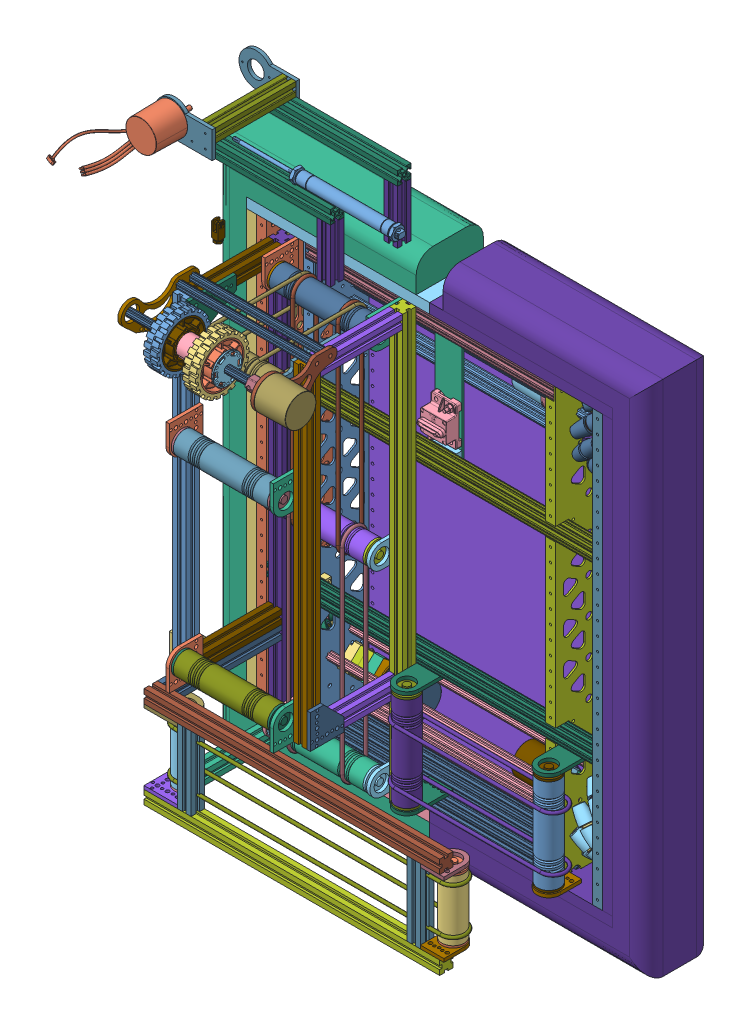
SolidWorks assembly Robot 2020, configuration Default. Lengths in mm.
Overall size (819.15 1227.35 564.02).
528 component instances, 164 part files, 0 mates.
Components (placement in the parent):
- Robot 2020(2)^Robot 2020-1: Robot 2020(2)^Robot 2020 [Default] at origin size (819.15 992.53 549) (virtual)
  - Fame 2020^Robot 2020(2)_Robot 2020-1: Fame 2020^Robot 2020(2)_Robot 2020 [Default] at origin size (819.15 977.9 171.99) (virtual)
    - Inner plate v12(Mirror)^Fame 2020_Robot 2020(2)_Robot 2020-1: Inner plate v12(Mirror)^Fame 2020_Robot 2020(2)_Robot 2020 [Default] at (-212.725 0 58.7875) x (0 1 0) z (0 0 -1) size (812.8 19.05 127) (virtual)
      - Inner plate v12(Mirror)-0^Inner plate v12(Mirror)_Fame 2020_Robot 2020(2)_Robot 2020-1: Inner plate v12(Mirror)-0^Inner plate v12(Mirror)_Fame 2020_Robot 2020(2)_Robot 2020 [Default] at origin size (812.8 19.05 127) (virtual)
    - Outer plate v11(Mirror)^Fame 2020_Robot 2020(2)_Robot 2020-1: Outer plate v11(Mirror)^Fame 2020_Robot 2020(2)_Robot 2020 [Default] at (-333.375 0 58.7875) x (0 -1 0) z (0 0 -1) size (812.8 19.05 127) (virtual)
      - Outer plate v11(Mirror)-1^Outer plate v11(Mirror)_Fame 2020_Robot 2020(2)_Robot 2020-1: Outer plate v11(Mirror)-1^Outer plate v11(Mirror)_Fame 2020_Robot 2020(2)_Robot 2020 [Default] at origin size (812.8 19.05 127) (virtual)
    - Bumper Assembly v4(Mirror)^Fame 2020_Robot 2020(2)_Robot 2020-1: Bumper Assembly v4(Mirror)^Fame 2020_Robot 2020(2)_Robot 2020 [Default] at (-327.025 0.0665 58.7875) x (-1 0 0) z (0 0 -1) size (409.58 977.9 127) (virtual)
      - Bumper Assembly v4(Mirror)-2^Bumper Assembly v4(Mirror)_Fame 2020_Robot 2020(2)_Robot 2020-1: Bumper Assembly v4(Mirror)-2^Bumper Assembly v4(Mirror)_Fame 2020_Robot 2020(2)_Robot 2020 [Default] at origin size (19.05 812.8 127) (virtual)
      - Bumper Assembly v4(Mirror)-3^Bumper Assembly v4(Mirror)_Fame 2020_Robot 2020(2)_Robot 2020-1: Bumper Assembly v4(Mirror)-3^Bumper Assembly v4(Mirror)_Fame 2020_Robot 2020(2)_Robot 2020 [Default] at origin size (346.08 19.05 127) (virtual)
      - Bumper Assembly v4(Mirror)-4^Bumper Assembly v4(Mirror)_Fame 2020_Robot 2020(2)_Robot 2020-1: Bumper Assembly v4(Mirror)-4^Bumper Assembly v4(Mirror)_Fame 2020_Robot 2020(2)_Robot 2020 [Default] at origin size (346.08 19.05 127) (virtual)
      - Bumper Assembly v4(Mirror)-5^Bumper Assembly v4(Mirror)_Fame 2020_Robot 2020(2)_Robot 2020-1: Bumper Assembly v4(Mirror)-5^Bumper Assembly v4(Mirror)_Fame 2020_Robot 2020(2)_Robot 2020 [Default] at origin size (409.58 977.9 127) (virtual)
    - NEO Gearbox 2-stage Custom^Fame 2020_Robot 2020(2)_Robot 2020-1: NEO Gearbox 2-stage Custom^Fame 2020_Robot 2020(2)_Robot 2020 [Default] at (0 0 425) size (164.9 90.53 90.53) (virtual)
      - VersaPlanetary_4_1_Gear_Kit_217-2818^NEO Gearbox 2-stage Custom_Fame 2020_Robot 2020(2)_Robot 2020-1: VersaPlanetary_4_1_Gear_Kit_217-2818^NEO Gearbox 2-stage Custom_Fame 2020_Robot 2020(2)_Robot 2020 [Default] at (-15.25 22.225 0) x (0 -0.707107 0.707107) z (-1 0 0) size (35.49 35.49 17.4) (virtual)
        - 217-2725-001 Rev1_24t Sun^VersaPlanetary_4_1_Gear_Kit_217-2818_NEO Gearbox 2-stage Custom_Fame 2020_Robot 2020(2)_Robot 2020-1: 217-2725-001 Rev1_24t Sun^VersaPlanetary_4_1_Gear_Kit_217-2818_NEO Gearbox 2-stage Custom_Fame 2020_Robot 2020(2)_Robot 2020 [Default] at (-36.69 -517.1337 -209.675) x (0.707107 0.707107 0) z (0 0 1) size (14.4 14.45 12.7) (virtual)
        - 217-2725-002 Rev1_24t Planet^VersaPlanetary_4_1_Gear_Kit_217-2818_NEO Gearbox 2-stage Custom_Fame 2020_Robot 2020(2)_Robot 2020-1: 217-2725-002 Rev1_24t Planet^VersaPlanetary_4_1_Gear_Kit_217-2818_NEO Gearbox 2-stage Custom_Fame 2020_Robot 2020(2)_Robot 2020 [Default] at (-45.2382 -525.6819 -212.025) x (-0.793353 0.608761 0) z (0 0 -1) size (13.12 13.1 8) (virtual)
        - 217-2724-002 Rev1^VersaPlanetary_4_1_Gear_Kit_217-2818_NEO Gearbox 2-stage Custom_Fame 2020_Robot 2020(2)_Robot 2020-1: 217-2724-002 Rev1^VersaPlanetary_4_1_Gear_Kit_217-2818_NEO Gearbox 2-stage Custom_Fame 2020_Robot 2020(2)_Robot 2020 [Default] at (-36.69 -517.1337 -218.375) x (1 0 0) z (0 0 -1) size (34.7 34.7 4.7) (virtual)
        - 217-2625-010 Rev1^VersaPlanetary_4_1_Gear_Kit_217-2818_NEO Gearbox 2-stage Custom_Fame 2020_Robot 2020(2)_Robot 2020-1: 217-2625-010 Rev1^VersaPlanetary_4_1_Gear_Kit_217-2818_NEO Gearbox 2-stage Custom_Fame 2020_Robot 2020(2)_Robot 2020 [Default] at (-45.2382 -525.6819 -214.725) x (0.854322 0.519745 0) z (0 0 1) size (4 4 12) (virtual)
        - 217-2725-002 Rev1_24t Planet^VersaPlanetary_4_1_Gear_Kit_217-2818_NEO Gearbox 2-stage Custom_Fame 2020_Robot 2020(2)_Robot 2020-2: 217-2725-002 Rev1_24t Planet^VersaPlanetary_4_1_Gear_Kit_217-2818_NEO Gearbox 2-stage Custom_Fame 2020_Robot 2020(2)_Robot 2020 [Default] at (-28.1418 -525.6819 -212.025) x (-0.608761 -0.793353 0) z (0 0 -1) size (13.12 13.1 8) (virtual)
        - 217-2725-002 Rev1_24t Planet^VersaPlanetary_4_1_Gear_Kit_217-2818_NEO Gearbox 2-stage Custom_Fame 2020_Robot 2020(2)_Robot 2020-3: 217-2725-002 Rev1_24t Planet^VersaPlanetary_4_1_Gear_Kit_217-2818_NEO Gearbox 2-stage Custom_Fame 2020_Robot 2020(2)_Robot 2020 [Default] at (-28.1418 -508.5855 -212.025) x (0.793353 -0.608761 0) z (0 0 -1) size (13.12 13.1 8) (virtual)
        - 217-2725-002 Rev1_24t Planet^VersaPlanetary_4_1_Gear_Kit_217-2818_NEO Gearbox 2-stage Custom_Fame 2020_Robot 2020(2)_Robot 2020-4: 217-2725-002 Rev1_24t Planet^VersaPlanetary_4_1_Gear_Kit_217-2818_NEO Gearbox 2-stage Custom_Fame 2020_Robot 2020(2)_Robot 2020 [Default] at (-45.2382 -508.5855 -212.025) x (0.608761 0.793353 0) z (0 0 -1) size (13.12 13.1 8) (virtual)
        - 217-2625-010 Rev1^VersaPlanetary_4_1_Gear_Kit_217-2818_NEO Gearbox 2-stage Custom_Fame 2020_Robot 2020(2)_Robot 2020-2: 217-2625-010 Rev1^VersaPlanetary_4_1_Gear_Kit_217-2818_NEO Gearbox 2-stage Custom_Fame 2020_Robot 2020(2)_Robot 2020 [Default] at (-28.1418 -525.6819 -214.725) x (-0.519745 0.854322 0) z (0 0 1) size (4 4 12) (virtual)
        - 217-2625-010 Rev1^VersaPlanetary_4_1_Gear_Kit_217-2818_NEO Gearbox 2-stage Custom_Fame 2020_Robot 2020(2)_Robot 2020-3: 217-2625-010 Rev1^VersaPlanetary_4_1_Gear_Kit_217-2818_NEO Gearbox 2-stage Custom_Fame 2020_Robot 2020(2)_Robot 2020 [Default] at (-28.1418 -508.5855 -214.725) x (-0.854322 -0.519745 0) z (0 0 1) size (4 4 12) (virtual)
        - 217-2625-010 Rev1^VersaPlanetary_4_1_Gear_Kit_217-2818_NEO Gearbox 2-stage Custom_Fame 2020_Robot 2020(2)_Robot 2020-4: 217-2625-010 Rev1^VersaPlanetary_4_1_Gear_Kit_217-2818_NEO Gearbox 2-stage Custom_Fame 2020_Robot 2020(2)_Robot 2020 [Default] at (-45.2382 -508.5855 -214.725) x (0.519745 -0.854322 0) z (0 0 1) size (4 4 12) (virtual)
      - 217-2625-026 Rev1^NEO Gearbox 2-stage Custom_Fame 2020_Robot 2020(2)_Robot 2020-1: 217-2625-026 Rev1^NEO Gearbox 2-stage Custom_Fame 2020_Robot 2020(2)_Robot 2020 [Default] at (211.875 -317.5 -391.6125) x (0 -0.707107 0.707107) z (-1 0 0) size (44.45 42 18.12) (virtual)
      - 217-2742-001 Rev4^NEO Gearbox 2-stage Custom_Fame 2020_Robot 2020(2)_Robot 2020-1: 217-2742-001 Rev4^NEO Gearbox 2-stage Custom_Fame 2020_Robot 2020(2)_Robot 2020 [Default] at (218.5752 -317.5 -391.6125) x (1 0 0) z (0 0.63857 0.769564) size (7 28 28) (virtual)
      - 217-2742-001 Rev4^NEO Gearbox 2-stage Custom_Fame 2020_Robot 2020(2)_Robot 2020-2: 217-2742-001 Rev4^NEO Gearbox 2-stage Custom_Fame 2020_Robot 2020(2)_Robot 2020 [Default] at (226.5752 -317.5 -391.6125) x (1 0 0) z (0 0.707107 0.707107) size (7 28 28) (virtual)
      - 217-2625-017 Rev1_9714K61^NEO Gearbox 2-stage Custom_Fame 2020_Robot 2020(2)_Robot 2020-1: 217-2625-017 Rev1_9714K61^NEO Gearbox 2-stage Custom_Fame 2020_Robot 2020(2)_Robot 2020 [Default] at (225.795 -317.6887 -391.9075) x (0 0.983393 0.181491) z (0 -0.181491 0.983393) size (28.51 4.98 27.43) (virtual)
      - 217-2625-025 Rev1^NEO Gearbox 2-stage Custom_Fame 2020_Robot 2020(2)_Robot 2020-1: 217-2625-025 Rev1^NEO Gearbox 2-stage Custom_Fame 2020_Robot 2020(2)_Robot 2020 [Default] at (182.475 -317.5 -391.6125) x (0 -0.707107 0.707107) z (-1 0 0) size (44.45 42 18) (virtual)
      - 217-2816-001 Rev1^NEO Gearbox 2-stage Custom_Fame 2020_Robot 2020(2)_Robot 2020-1: 217-2816-001 Rev1^NEO Gearbox 2-stage Custom_Fame 2020_Robot 2020(2)_Robot 2020 [Default] at (212.025 -317.5 -391.6125) x (0 -0.707107 0.707107) z (1 0 0) size (42 42 14.5) (virtual)
      - 217-2816-001 Rev1^NEO Gearbox 2-stage Custom_Fame 2020_Robot 2020(2)_Robot 2020-2: 217-2816-001 Rev1^NEO Gearbox 2-stage Custom_Fame 2020_Robot 2020(2)_Robot 2020 [Default] at (199.325 -317.5 -391.6125) x (0 -0.707107 0.707107) z (1 0 0) size (42 42 14.5) (virtual)
      - 217-4649-001 Rev1^NEO Gearbox 2-stage Custom_Fame 2020_Robot 2020(2)_Robot 2020-1: 217-4649-001 Rev1^NEO Gearbox 2-stage Custom_Fame 2020_Robot 2020(2)_Robot 2020 [Default] at (185.629 -317.5 -391.6125) x (0 -0.707107 0.707107) z (1 0 0) size (18 18 13) (virtual)
      - VersaPlanetary_CIM_Adapter_217-4018^NEO Gearbox 2-stage Custom_Fame 2020_Robot 2020(2)_Robot 2020-1: VersaPlanetary_CIM_Adapter_217-4018^NEO Gearbox 2-stage Custom_Fame 2020_Robot 2020(2)_Robot 2020 [Default] at (165.15 -317.5 -391.6125) x (0 -0.707107 0.707107) z (0 0.707107 0.707107) size (64.01 21.55 64.01) (virtual)
      - NEO Motor REV-21-1650^NEO Gearbox 2-stage Custom_Fame 2020_Robot 2020(2)_Robot 2020-1: NEO Motor REV-21-1650^NEO Gearbox 2-stage Custom_Fame 2020_Robot 2020(2)_Robot 2020 [Default] at (153.625 -317.5 -391.6125) x (0 -0.707107 -0.707107) z (1 0 0) size (61.14 61.02 93.25) (virtual)
      - 3_1 Output Shaft Custom^NEO Gearbox 2-stage Custom_Fame 2020_Robot 2020(2)_Robot 2020-1: 3_1 Output Shaft Custom^NEO Gearbox 2-stage Custom_Fame 2020_Robot 2020(2)_Robot 2020 [Default] at (211.3752 -317.5 -391.6125) x (1 0 0) z (0 0.707107 0.707107) size (48.9 34.7 34.7) (virtual)
    - Left Wheel Assembly^Fame 2020_Robot 2020(2)_Robot 2020-1: Left Wheel Assembly^Fame 2020_Robot 2020(2)_Robot 2020 [Default] at (500 0 0) size (65.82 166.11 165.01) (virtual)
      - 6_Mecanum_Wheel_Left_217-2799^Left Wheel Assembly_Fame 2020_Robot 2020(2)_Robot 2020-1: 6_Mecanum_Wheel_Left_217-2799^Left Wheel Assembly_Fame 2020_Robot 2020(2)_Robot 2020 [Default] x (0 0 1) z (-1 0 0) size (165.01 166.11 65.82) (virtual)
        - 217-2799-001 Rev1^6_Mecanum_Wheel_Left_217-2799_Left Wheel Assembly_Fame 2020_Robot 2020(2)_Robot 2020-1: 217-2799-001 Rev1^6_Mecanum_Wheel_Left_217-2799_Left Wheel Assembly_Fame 2020_Robot 2020(2)_Robot 2020 [Default] at (33.3875 -317.5 234.0098) x (0.707107 0.707107 0) z (0 0 1) size (95.78 100.46 28.55) (virtual)
        - 217-2799-001 Rev1^6_Mecanum_Wheel_Left_217-2799_Left Wheel Assembly_Fame 2020_Robot 2020(2)_Robot 2020-2: 217-2799-001 Rev1^6_Mecanum_Wheel_Left_217-2799_Left Wheel Assembly_Fame 2020_Robot 2020(2)_Robot 2020 [Default] at (33.3875 -317.5 221.3098) x (-0.987688 -0.156434 0) z (0 0 -1) size (95.78 100.46 28.55) (virtual)
        - 217-2799-002 Rev1^6_Mecanum_Wheel_Left_217-2799_Left Wheel Assembly_Fame 2020_Robot 2020(2)_Robot 2020-1: 217-2799-002 Rev1^6_Mecanum_Wheel_Left_217-2799_Left Wheel Assembly_Fame 2020_Robot 2020(2)_Robot 2020 [Default] at (4.057 -346.8305 227.6598) x (-0.707107 0.707107 0) z (-0.707107 -0.707107 0) size (26.84 25.39 30.1) (virtual)
        - 217-2586-003 Rev2^6_Mecanum_Wheel_Left_217-2799_Left Wheel Assembly_Fame 2020_Robot 2020(2)_Robot 2020-1: 217-2586-003 Rev2^6_Mecanum_Wheel_Left_217-2799_Left Wheel Assembly_Fame 2020_Robot 2020(2)_Robot 2020 [Default] at (-13.4676 -358.6894 223.6536) x (0.41944 0.854155 0.30739) z (-0.757674 0.142894 0.636798) size (19.46 28.57 19.46) (virtual)
        - 217-2586-003 Rev2^6_Mecanum_Wheel_Left_217-2799_Left Wheel Assembly_Fame 2020_Robot 2020(2)_Robot 2020-2: 217-2586-003 Rev2^6_Mecanum_Wheel_Left_217-2799_Left Wheel Assembly_Fame 2020_Robot 2020(2)_Robot 2020 [Default] at (-7.8019 -364.3551 231.666) x (0.847342 0.451134 -0.280161) z (0.17892 -0.739241 -0.649238) size (19.46 28.57 19.46) (virtual)
        - 217-2586-004 Rev1^6_Mecanum_Wheel_Left_217-2799_Left Wheel Assembly_Fame 2020_Robot 2020(2)_Robot 2020-1: 217-2586-004 Rev1^6_Mecanum_Wheel_Left_217-2799_Left Wheel Assembly_Fame 2020_Robot 2020(2)_Robot 2020 [Default] at (-10.3479 -361.809 228.0654) x (-0.690521 -0.722949 -0.02293) z (0.522667 -0.476807 -0.706735) size (25.9 28.58 25.9) (virtual)
        - 217-2586-004 Rev1^6_Mecanum_Wheel_Left_217-2799_Left Wheel Assembly_Fame 2020_Robot 2020(2)_Robot 2020-2: 217-2586-004 Rev1^6_Mecanum_Wheel_Left_217-2799_Left Wheel Assembly_Fame 2020_Robot 2020(2)_Robot 2020 [Default] at (-10.9209 -361.2361 227.2551) x (0.01458 -0.811521 -0.584142) z (-0.865903 -0.302381 0.39847) size (25.9 28.58 25.9) (virtual)
        - 217-2586-007 Rev1^6_Mecanum_Wheel_Left_217-2799_Left Wheel Assembly_Fame 2020_Robot 2020(2)_Robot 2020-1: 217-2586-007 Rev1^6_Mecanum_Wheel_Left_217-2799_Left Wheel Assembly_Fame 2020_Robot 2020(2)_Robot 2020 [Default] at (-10.6347 -361.5222 227.6598) x (0.5 -0.5 0.707107) z (-0.709055 -0.705148 0.002763) size (61.72 5 5) (virtual)
        - 217-2586-008 Rev1^6_Mecanum_Wheel_Left_217-2799_Left Wheel Assembly_Fame 2020_Robot 2020(2)_Robot 2020-1: 217-2586-008 Rev1^6_Mecanum_Wheel_Left_217-2799_Left Wheel Assembly_Fame 2020_Robot 2020(2)_Robot 2020 [Default] at (53.3583 -330.4692 227.5328) x (0.544639 0.838671 0) z (0 0 -1) size (7.33 6.35 31.75) (virtual)
        - NUT-832-NYLOCK^6_Mecanum_Wheel_Left_217-2799_Left Wheel Assembly_Fame 2020_Robot 2020(2)_Robot 2020-1: NUT-832-NYLOCK^6_Mecanum_Wheel_Left_217-2799_Left Wheel Assembly_Fame 2020_Robot 2020(2)_Robot 2020 [Default] at (6.1639 -290.2764 241.3161) x (0.258819 -0.965926 0) z (-0.965926 -0.258819 0) size (9.37 5.86 8.12) (virtual)
        - SCREW-832-1250^6_Mecanum_Wheel_Left_217-2799_Left Wheel Assembly_Fame 2020_Robot 2020(2)_Robot 2020-1: SCREW-832-1250^6_Mecanum_Wheel_Left_217-2799_Left Wheel Assembly_Fame 2020_Robot 2020(2)_Robot 2020 [Default] at (6.1639 -290.2764 212.75) x (0 0 1) z (-0.394243 0.919006 0) size (33.96 7.92 7.92) (virtual)
        - 217-2586-007 Rev1^6_Mecanum_Wheel_Left_217-2799_Left Wheel Assembly_Fame 2020_Robot 2020(2)_Robot 2020-2: 217-2586-007 Rev1^6_Mecanum_Wheel_Left_217-2799_Left Wheel Assembly_Fame 2020_Robot 2020(2)_Robot 2020 [Default] at (-28.1029 -327.2391 227.6598) x (0.110616 -0.698401 0.707107) z (-0.988113 -0.153705 0.002763) size (61.72 5 5) (virtual)
        - 217-2586-007 Rev1^6_Mecanum_Wheel_Left_217-2799_Left Wheel Assembly_Fame 2020_Robot 2020(2)_Robot 2020-3: 217-2586-007 Rev1^6_Mecanum_Wheel_Left_217-2799_Left Wheel Assembly_Fame 2020_Robot 2020(2)_Robot 2020 [Default] at (-22.0838 -289.236 227.6598) x (-0.32102 -0.630037 0.707107) z (-0.889746 0.456448 0.002763) size (61.72 5 5) (virtual)
        - 217-2586-007 Rev1^6_Mecanum_Wheel_Left_217-2799_Left Wheel Assembly_Fame 2020_Robot 2020(2)_Robot 2020-4: 217-2586-007 Rev1^6_Mecanum_Wheel_Left_217-2799_Left Wheel Assembly_Fame 2020_Robot 2020(2)_Robot 2020 [Default] at (5.1235 -262.0287 227.6598) x (-0.630037 -0.32102 0.707107) z (-0.451526 0.892254 0.002763) size (61.72 5 5) (virtual)
        - 217-2586-007 Rev1^6_Mecanum_Wheel_Left_217-2799_Left Wheel Assembly_Fame 2020_Robot 2020(2)_Robot 2020-5: 217-2586-007 Rev1^6_Mecanum_Wheel_Left_217-2799_Left Wheel Assembly_Fame 2020_Robot 2020(2)_Robot 2020 [Default] at (43.1266 -256.0096 227.6598) x (-0.698401 0.110616 0.707107) z (0.159162 0.987249 0.002763) size (61.72 5 5) (virtual)
        - 217-2586-007 Rev1^6_Mecanum_Wheel_Left_217-2799_Left Wheel Assembly_Fame 2020_Robot 2020(2)_Robot 2020-6: 217-2586-007 Rev1^6_Mecanum_Wheel_Left_217-2799_Left Wheel Assembly_Fame 2020_Robot 2020(2)_Robot 2020 [Default] at (77.4097 -273.4778 227.6598) x (-0.5 0.5 0.707107) z (0.709055 0.705148 0.002763) size (61.72 5 5) (virtual)
        - 217-2586-007 Rev1^6_Mecanum_Wheel_Left_217-2799_Left Wheel Assembly_Fame 2020_Robot 2020(2)_Robot 2020-7: 217-2586-007 Rev1^6_Mecanum_Wheel_Left_217-2799_Left Wheel Assembly_Fame 2020_Robot 2020(2)_Robot 2020 [Default] at (94.8779 -307.7609 227.6598) x (-0.110616 0.698401 0.707107) z (0.988113 0.153705 0.002763) size (61.72 5 5) (virtual)
        - 217-2586-007 Rev1^6_Mecanum_Wheel_Left_217-2799_Left Wheel Assembly_Fame 2020_Robot 2020(2)_Robot 2020-8: 217-2586-007 Rev1^6_Mecanum_Wheel_Left_217-2799_Left Wheel Assembly_Fame 2020_Robot 2020(2)_Robot 2020 [Default] at (88.8588 -345.764 227.6598) x (0.32102 0.630037 0.707107) z (0.889746 -0.456448 0.002763) size (61.72 5 5) (virtual)
        - 217-2586-007 Rev1^6_Mecanum_Wheel_Left_217-2799_Left Wheel Assembly_Fame 2020_Robot 2020(2)_Robot 2020-9: 217-2586-007 Rev1^6_Mecanum_Wheel_Left_217-2799_Left Wheel Assembly_Fame 2020_Robot 2020(2)_Robot 2020 [Default] at (61.6515 -372.9713 227.6598) x (0.630037 0.32102 0.707107) z (0.451526 -0.892254 0.002763) size (61.72 5 5) (virtual)
        - 217-2586-007 Rev1^6_Mecanum_Wheel_Left_217-2799_Left Wheel Assembly_Fame 2020_Robot 2020(2)_Robot 2020-10: 217-2586-007 Rev1^6_Mecanum_Wheel_Left_217-2799_Left Wheel Assembly_Fame 2020_Robot 2020(2)_Robot 2020 [Default] at (23.6484 -378.9904 227.6598) x (0.698401 -0.110616 0.707107) z (-0.159162 -0.987249 0.002763) size (61.72 5 5) (virtual)
        - 217-2586-004 Rev1^6_Mecanum_Wheel_Left_217-2799_Left Wheel Assembly_Fame 2020_Robot 2020(2)_Robot 2020-3: 217-2586-004 Rev1^6_Mecanum_Wheel_Left_217-2799_Left Wheel Assembly_Fame 2020_Robot 2020(2)_Robot 2020 [Default] at (-28.1662 -326.8394 227.2551) x (-0.465204 -0.665104 -0.584142) z (-0.878265 0.264334 0.39847) size (25.9 28.58 25.9) (virtual)
        - 217-2586-004 Rev1^6_Mecanum_Wheel_Left_217-2799_Left Wheel Assembly_Fame 2020_Robot 2020(2)_Robot 2020-4: 217-2586-004 Rev1^6_Mecanum_Wheel_Left_217-2799_Left Wheel Assembly_Fame 2020_Robot 2020(2)_Robot 2020 [Default] at (-21.9 -288.8754 227.2551) x (-0.767297 -0.26464 -0.584142) z (-0.55516 0.730082 0.39847) size (25.9 28.58 25.9) (virtual)
        - 217-2586-004 Rev1^6_Mecanum_Wheel_Left_217-2799_Left Wheel Assembly_Fame 2020_Robot 2020(2)_Robot 2020-5: 217-2586-004 Rev1^6_Mecanum_Wheel_Left_217-2799_Left Wheel Assembly_Fame 2020_Robot 2020(2)_Robot 2020 [Default] at (5.484 -261.845 227.2551) x (-0.776308 0.236907 -0.584142) z (-0.020002 0.916963 0.39847) size (25.9 28.58 25.9) (virtual)
        - 217-2586-004 Rev1^6_Mecanum_Wheel_Left_217-2799_Left Wheel Assembly_Fame 2020_Robot 2020(2)_Robot 2020-6: 217-2586-004 Rev1^6_Mecanum_Wheel_Left_217-2799_Left Wheel Assembly_Fame 2020_Robot 2020(2)_Robot 2020 [Default] at (43.5263 -256.0729 227.2551) x (-0.488796 0.647964 -0.584142) z (0.522795 0.753596 0.39847) size (25.9 28.58 25.9) (virtual)
        - 217-2586-004 Rev1^6_Mecanum_Wheel_Left_217-2799_Left Wheel Assembly_Fame 2020_Robot 2020(2)_Robot 2020-7: 217-2586-004 Rev1^6_Mecanum_Wheel_Left_217-2799_Left Wheel Assembly_Fame 2020_Robot 2020(2)_Robot 2020 [Default] at (77.6959 -273.7639 227.2551) x (-0.01458 0.811521 -0.584142) z (0.865903 0.302381 0.39847) size (25.9 28.58 25.9) (virtual)
        - 217-2586-004 Rev1^6_Mecanum_Wheel_Left_217-2799_Left Wheel Assembly_Fame 2020_Robot 2020(2)_Robot 2020-8: 217-2586-004 Rev1^6_Mecanum_Wheel_Left_217-2799_Left Wheel Assembly_Fame 2020_Robot 2020(2)_Robot 2020 [Default] at (94.9412 -308.1606 227.2551) x (0.465204 0.665104 -0.584142) z (0.878265 -0.264334 0.39847) size (25.9 28.58 25.9) (virtual)
        - 217-2586-004 Rev1^6_Mecanum_Wheel_Left_217-2799_Left Wheel Assembly_Fame 2020_Robot 2020(2)_Robot 2020-9: 217-2586-004 Rev1^6_Mecanum_Wheel_Left_217-2799_Left Wheel Assembly_Fame 2020_Robot 2020(2)_Robot 2020 [Default] at (88.675 -346.1246 227.2551) x (0.767297 0.26464 -0.584142) z (0.55516 -0.730082 0.39847) size (25.9 28.58 25.9) (virtual)
        - 217-2586-004 Rev1^6_Mecanum_Wheel_Left_217-2799_Left Wheel Assembly_Fame 2020_Robot 2020(2)_Robot 2020-10: 217-2586-004 Rev1^6_Mecanum_Wheel_Left_217-2799_Left Wheel Assembly_Fame 2020_Robot 2020(2)_Robot 2020 [Default] at (61.291 -373.155 227.2551) x (0.776308 -0.236907 -0.584142) z (0.020002 -0.916963 0.39847) size (25.9 28.58 25.9) (virtual)
        - 217-2586-004 Rev1^6_Mecanum_Wheel_Left_217-2799_Left Wheel Assembly_Fame 2020_Robot 2020(2)_Robot 2020-11: 217-2586-004 Rev1^6_Mecanum_Wheel_Left_217-2799_Left Wheel Assembly_Fame 2020_Robot 2020(2)_Robot 2020 [Default] at (23.2487 -378.9271 227.2551) x (0.488796 -0.647964 -0.584142) z (-0.522795 -0.753596 0.39847) size (25.9 28.58 25.9) (virtual)
        - 217-2586-004 Rev1^6_Mecanum_Wheel_Left_217-2799_Left Wheel Assembly_Fame 2020_Robot 2020(2)_Robot 2020-12: 217-2586-004 Rev1^6_Mecanum_Wheel_Left_217-2799_Left Wheel Assembly_Fame 2020_Robot 2020(2)_Robot 2020 [Default] at (-28.0394 -327.6397 228.0654) x (-0.983582 -0.179 -0.02293) z (0.142587 -0.692961 -0.706735) size (25.9 28.58 25.9) (virtual)
        - 217-2586-004 Rev1^6_Mecanum_Wheel_Left_217-2799_Left Wheel Assembly_Fame 2020_Robot 2020(2)_Robot 2020-13: 217-2586-004 Rev1^6_Mecanum_Wheel_Left_217-2799_Left Wheel Assembly_Fame 2020_Robot 2020(2)_Robot 2020 [Default] at (-22.2679 -289.5974 228.0654) x (-0.900948 0.433321 -0.02293) z (-0.291957 -0.644427 -0.706735) size (25.9 28.58 25.9) (virtual)
        - 217-2586-004 Rev1^6_Mecanum_Wheel_Left_217-2799_Left Wheel Assembly_Fame 2020_Robot 2020(2)_Robot 2020-14: 217-2586-004 Rev1^6_Mecanum_Wheel_Left_217-2799_Left Wheel Assembly_Fame 2020_Robot 2020(2)_Robot 2020 [Default] at (4.7621 -262.2129 228.0654) x (-0.474183 0.880128 -0.02293) z (-0.614983 -0.349745 -0.706735) size (25.9 28.58 25.9) (virtual)
        - 217-2586-004 Rev1^6_Mecanum_Wheel_Left_217-2799_Left Wheel Assembly_Fame 2020_Robot 2020(2)_Robot 2020-15: 217-2586-004 Rev1^6_Mecanum_Wheel_Left_217-2799_Left Wheel Assembly_Fame 2020_Robot 2020(2)_Robot 2020 [Default] at (42.726 -255.9462 228.0654) x (0.133704 0.990756 -0.02293) z (-0.703107 0.078529 -0.706735) size (25.9 28.58 25.9) (virtual)
        - 217-2586-004 Rev1^6_Mecanum_Wheel_Left_217-2799_Left Wheel Assembly_Fame 2020_Robot 2020(2)_Robot 2020-16: 217-2586-004 Rev1^6_Mecanum_Wheel_Left_217-2799_Left Wheel Assembly_Fame 2020_Robot 2020(2)_Robot 2020 [Default] at (77.1229 -273.191 228.0654) x (0.690521 0.722949 -0.02293) z (-0.522667 0.476807 -0.706735) size (25.9 28.58 25.9) (virtual)
        - 217-2586-004 Rev1^6_Mecanum_Wheel_Left_217-2799_Left Wheel Assembly_Fame 2020_Robot 2020(2)_Robot 2020-17: 217-2586-004 Rev1^6_Mecanum_Wheel_Left_217-2799_Left Wheel Assembly_Fame 2020_Robot 2020(2)_Robot 2020 [Default] at (94.8144 -307.3603 228.0654) x (0.983582 0.179 -0.02293) z (-0.142587 0.692961 -0.706735) size (25.9 28.58 25.9) (virtual)
        - 217-2586-004 Rev1^6_Mecanum_Wheel_Left_217-2799_Left Wheel Assembly_Fame 2020_Robot 2020(2)_Robot 2020-18: 217-2586-004 Rev1^6_Mecanum_Wheel_Left_217-2799_Left Wheel Assembly_Fame 2020_Robot 2020(2)_Robot 2020 [Default] at (89.0429 -345.4026 228.0654) x (0.900948 -0.433321 -0.02293) z (0.291957 0.644427 -0.706735) size (25.9 28.58 25.9) (virtual)
        - 217-2586-004 Rev1^6_Mecanum_Wheel_Left_217-2799_Left Wheel Assembly_Fame 2020_Robot 2020(2)_Robot 2020-19: 217-2586-004 Rev1^6_Mecanum_Wheel_Left_217-2799_Left Wheel Assembly_Fame 2020_Robot 2020(2)_Robot 2020 [Default] at (62.0129 -372.7871 228.0654) x (0.474183 -0.880128 -0.02293) z (0.614983 0.349745 -0.706735) size (25.9 28.58 25.9) (virtual)
        - 217-2586-004 Rev1^6_Mecanum_Wheel_Left_217-2799_Left Wheel Assembly_Fame 2020_Robot 2020(2)_Robot 2020-20: 217-2586-004 Rev1^6_Mecanum_Wheel_Left_217-2799_Left Wheel Assembly_Fame 2020_Robot 2020(2)_Robot 2020 [Default] at (24.049 -379.0538 228.0654) x (-0.133704 -0.990756 -0.02293) z (0.703107 -0.078529 -0.706735) size (25.9 28.58 25.9) (virtual)
        - 217-2586-003 Rev2^6_Mecanum_Wheel_Left_217-2799_Left Wheel Assembly_Fame 2020_Robot 2020(2)_Robot 2020-3: 217-2586-003 Rev2^6_Mecanum_Wheel_Left_217-2799_Left Wheel Assembly_Fame 2020_Robot 2020(2)_Robot 2020 [Default] at (-27.4761 -331.196 231.666) x (0.950684 -0.13308 -0.280161) z (-0.289766 -0.703225 -0.649238) size (19.46 28.57 19.46) (virtual)
        - 217-2586-003 Rev2^6_Mecanum_Wheel_Left_217-2799_Left Wheel Assembly_Fame 2020_Robot 2020(2)_Robot 2020-4: 217-2586-003 Rev2^6_Mecanum_Wheel_Left_217-2799_Left Wheel Assembly_Fame 2020_Robot 2020(2)_Robot 2020 [Default] at (-23.9025 -292.8056 231.666) x (0.690897 -0.666462 -0.280161) z (-0.647771 -0.398601 -0.649238) size (19.46 28.57 19.46) (virtual)
        - 217-2586-003 Rev2^6_Mecanum_Wheel_Left_217-2799_Left Wheel Assembly_Fame 2020_Robot 2020(2)_Robot 2020-5: 217-2586-003 Rev2^6_Mecanum_Wheel_Left_217-2799_Left Wheel Assembly_Fame 2020_Robot 2020(2)_Robot 2020 [Default] at (1.5539 -263.8475 231.666) x (0.167211 -0.945278 -0.280161) z (-0.75835 0.058276 -0.649238) size (19.46 28.57 19.46) (virtual)
        - 217-2586-003 Rev2^6_Mecanum_Wheel_Left_217-2799_Left Wheel Assembly_Fame 2020_Robot 2020(2)_Robot 2020-6: 217-2586-003 Rev2^6_Mecanum_Wheel_Left_217-2799_Left Wheel Assembly_Fame 2020_Robot 2020(2)_Robot 2020 [Default] at (39.1697 -255.3829 231.666) x (-0.420344 -0.86303 -0.280161) z (-0.579264 0.492893 -0.649238) size (19.46 28.57 19.46) (virtual)
        - 217-2586-003 Rev2^6_Mecanum_Wheel_Left_217-2799_Left Wheel Assembly_Fame 2020_Robot 2020(2)_Robot 2020-7: 217-2586-003 Rev2^6_Mecanum_Wheel_Left_217-2799_Left Wheel Assembly_Fame 2020_Robot 2020(2)_Robot 2020 [Default] at (74.5769 -270.6449 231.666) x (-0.847342 -0.451134 -0.280161) z (-0.17892 0.739241 -0.649238) size (19.46 28.57 19.46) (virtual)
        - 217-2586-003 Rev2^6_Mecanum_Wheel_Left_217-2799_Left Wheel Assembly_Fame 2020_Robot 2020(2)_Robot 2020-8: 217-2586-003 Rev2^6_Mecanum_Wheel_Left_217-2799_Left Wheel Assembly_Fame 2020_Robot 2020(2)_Robot 2020 [Default] at (94.2511 -303.804 231.666) x (-0.950684 0.13308 -0.280161) z (0.289766 0.703225 -0.649238) size (19.46 28.57 19.46) (virtual)
        - 217-2586-003 Rev2^6_Mecanum_Wheel_Left_217-2799_Left Wheel Assembly_Fame 2020_Robot 2020(2)_Robot 2020-9: 217-2586-003 Rev2^6_Mecanum_Wheel_Left_217-2799_Left Wheel Assembly_Fame 2020_Robot 2020(2)_Robot 2020 [Default] at (90.6775 -342.1944 231.666) x (-0.690897 0.666462 -0.280161) z (0.647771 0.398601 -0.649238) size (19.46 28.57 19.46) (virtual)
        - 217-2586-003 Rev2^6_Mecanum_Wheel_Left_217-2799_Left Wheel Assembly_Fame 2020_Robot 2020(2)_Robot 2020-10: 217-2586-003 Rev2^6_Mecanum_Wheel_Left_217-2799_Left Wheel Assembly_Fame 2020_Robot 2020(2)_Robot 2020 [Default] at (65.2211 -371.1525 231.666) x (-0.167211 0.945278 -0.280161) z (0.75835 -0.058276 -0.649238) size (19.46 28.57 19.46) (virtual)
        - 217-2586-003 Rev2^6_Mecanum_Wheel_Left_217-2799_Left Wheel Assembly_Fame 2020_Robot 2020(2)_Robot 2020-11: 217-2586-003 Rev2^6_Mecanum_Wheel_Left_217-2799_Left Wheel Assembly_Fame 2020_Robot 2020(2)_Robot 2020 [Default] at (27.6053 -379.6171 231.666) x (0.420344 0.86303 -0.280161) z (0.579264 -0.492893 -0.649238) size (19.46 28.57 19.46) (virtual)
        - 217-2586-003 Rev2^6_Mecanum_Wheel_Left_217-2799_Left Wheel Assembly_Fame 2020_Robot 2020(2)_Robot 2020-12: 217-2586-003 Rev2^6_Mecanum_Wheel_Left_217-2799_Left Wheel Assembly_Fame 2020_Robot 2020(2)_Robot 2020 [Default] at (-28.7296 -323.2822 223.6536) x (0.841394 0.444485 0.30739) z (-0.52898 0.560953 0.636798) size (19.46 28.57 19.46) (virtual)
        - 217-2586-003 Rev2^6_Mecanum_Wheel_Left_217-2799_Left Wheel Assembly_Fame 2020_Robot 2020(2)_Robot 2020-13: 217-2586-003 Rev2^6_Mecanum_Wheel_Left_217-2799_Left Wheel Assembly_Fame 2020_Robot 2020(2)_Robot 2020 [Default] at (-20.265 -285.6664 223.6536) x (0.941964 -0.134963 0.30739) z (-0.098234 0.764747 0.636798) size (19.46 28.57 19.46) (virtual)
        - 217-2586-003 Rev2^6_Mecanum_Wheel_Left_217-2799_Left Wheel Assembly_Fame 2020_Robot 2020(2)_Robot 2020-14: 217-2586-003 Rev2^6_Mecanum_Wheel_Left_217-2799_Left Wheel Assembly_Fame 2020_Robot 2020(2)_Robot 2020 [Default] at (8.6931 -260.21 223.6536) x (0.682736 -0.66286 0.30739) z (0.370035 0.676434 0.636798) size (19.46 28.57 19.46) (virtual)
        - 217-2586-003 Rev2^6_Mecanum_Wheel_Left_217-2799_Left Wheel Assembly_Fame 2020_Robot 2020(2)_Robot 2020-15: 217-2586-003 Rev2^6_Mecanum_Wheel_Left_217-2799_Left Wheel Assembly_Fame 2020_Robot 2020(2)_Robot 2020 [Default] at (47.0835 -256.6364 223.6536) x (0.162726 -0.937567 0.30739) z (0.696962 0.329746 0.636798) size (19.46 28.57 19.46) (virtual)
        - 217-2586-003 Rev2^6_Mecanum_Wheel_Left_217-2799_Left Wheel Assembly_Fame 2020_Robot 2020(2)_Robot 2020-16: 217-2586-003 Rev2^6_Mecanum_Wheel_Left_217-2799_Left Wheel Assembly_Fame 2020_Robot 2020(2)_Robot 2020 [Default] at (80.2426 -276.3106 223.6536) x (-0.41944 -0.854155 0.30739) z (0.757674 -0.142894 0.636798) size (19.46 28.57 19.46) (virtual)
        - 217-2586-003 Rev2^6_Mecanum_Wheel_Left_217-2799_Left Wheel Assembly_Fame 2020_Robot 2020(2)_Robot 2020-17: 217-2586-003 Rev2^6_Mecanum_Wheel_Left_217-2799_Left Wheel Assembly_Fame 2020_Robot 2020(2)_Robot 2020 [Default] at (95.5046 -311.7178 223.6536) x (-0.841394 -0.444485 0.30739) z (0.52898 -0.560953 0.636798) size (19.46 28.57 19.46) (virtual)
        - 217-2586-003 Rev2^6_Mecanum_Wheel_Left_217-2799_Left Wheel Assembly_Fame 2020_Robot 2020(2)_Robot 2020-18: 217-2586-003 Rev2^6_Mecanum_Wheel_Left_217-2799_Left Wheel Assembly_Fame 2020_Robot 2020(2)_Robot 2020 [Default] at (87.04 -349.3336 223.6536) x (-0.941964 0.134963 0.30739) z (0.098234 -0.764747 0.636798) size (19.46 28.57 19.46) (virtual)
        - 217-2586-003 Rev2^6_Mecanum_Wheel_Left_217-2799_Left Wheel Assembly_Fame 2020_Robot 2020(2)_Robot 2020-19: 217-2586-003 Rev2^6_Mecanum_Wheel_Left_217-2799_Left Wheel Assembly_Fame 2020_Robot 2020(2)_Robot 2020 [Default] at (58.0819 -374.79 223.6536) x (-0.682736 0.66286 0.30739) z (-0.370035 -0.676434 0.636798) size (19.46 28.57 19.46) (virtual)
        - 217-2586-003 Rev2^6_Mecanum_Wheel_Left_217-2799_Left Wheel Assembly_Fame 2020_Robot 2020(2)_Robot 2020-20: 217-2586-003 Rev2^6_Mecanum_Wheel_Left_217-2799_Left Wheel Assembly_Fame 2020_Robot 2020(2)_Robot 2020 [Default] at (19.6915 -378.3636 223.6536) x (-0.162726 0.937567 0.30739) z (-0.696962 -0.329746 0.636798) size (19.46 28.57 19.46) (virtual)
        - 217-2799-002 Rev1^6_Mecanum_Wheel_Left_217-2799_Left Wheel Assembly_Fame 2020_Robot 2020(2)_Robot 2020-2: 217-2799-002 Rev1^6_Mecanum_Wheel_Left_217-2799_Left Wheel Assembly_Fame 2020_Robot 2020(2)_Robot 2020 [Default] at (-7.5815 -323.9888 227.6598) x (-0.156434 0.987688 0) z (-0.987688 -0.156434 0) size (26.84 25.39 30.1) (virtual)
        - 217-2799-002 Rev1^6_Mecanum_Wheel_Left_217-2799_Left Wheel Assembly_Fame 2020_Robot 2020(2)_Robot 2020-3: 217-2799-002 Rev1^6_Mecanum_Wheel_Left_217-2799_Left Wheel Assembly_Fame 2020_Robot 2020(2)_Robot 2020 [Default] at (-3.5711 -298.6686 227.6598) x (0.45399 0.891007 0) z (-0.891007 0.45399 0) size (26.84 25.39 30.1) (virtual)
        - 217-2799-002 Rev1^6_Mecanum_Wheel_Left_217-2799_Left Wheel Assembly_Fame 2020_Robot 2020(2)_Robot 2020-4: 217-2799-002 Rev1^6_Mecanum_Wheel_Left_217-2799_Left Wheel Assembly_Fame 2020_Robot 2020(2)_Robot 2020 [Default] at (14.5561 -280.5414 227.6598) x (0.891007 0.45399 0) z (-0.45399 0.891007 0) size (26.84 25.39 30.1) (virtual)
        - 217-2799-002 Rev1^6_Mecanum_Wheel_Left_217-2799_Left Wheel Assembly_Fame 2020_Robot 2020(2)_Robot 2020-5: 217-2799-002 Rev1^6_Mecanum_Wheel_Left_217-2799_Left Wheel Assembly_Fame 2020_Robot 2020(2)_Robot 2020 [Default] at (39.8763 -276.531 227.6598) x (0.987688 -0.156434 0) z (0.156434 0.987688 0) size (26.84 25.39 30.1) (virtual)
        - 217-2799-002 Rev1^6_Mecanum_Wheel_Left_217-2799_Left Wheel Assembly_Fame 2020_Robot 2020(2)_Robot 2020-6: 217-2799-002 Rev1^6_Mecanum_Wheel_Left_217-2799_Left Wheel Assembly_Fame 2020_Robot 2020(2)_Robot 2020 [Default] at (62.718 -288.1695 227.6598) x (0.707107 -0.707107 0) z (0.707107 0.707107 0) size (26.84 25.39 30.1) (virtual)
        - 217-2799-002 Rev1^6_Mecanum_Wheel_Left_217-2799_Left Wheel Assembly_Fame 2020_Robot 2020(2)_Robot 2020-7: 217-2799-002 Rev1^6_Mecanum_Wheel_Left_217-2799_Left Wheel Assembly_Fame 2020_Robot 2020(2)_Robot 2020 [Default] at (74.3565 -311.0112 227.6598) x (0.156434 -0.987688 0) z (0.987688 0.156434 0) size (26.84 25.39 30.1) (virtual)
        - 217-2799-002 Rev1^6_Mecanum_Wheel_Left_217-2799_Left Wheel Assembly_Fame 2020_Robot 2020(2)_Robot 2020-8: 217-2799-002 Rev1^6_Mecanum_Wheel_Left_217-2799_Left Wheel Assembly_Fame 2020_Robot 2020(2)_Robot 2020 [Default] at (70.3461 -336.3314 227.6598) x (-0.45399 -0.891007 0) z (0.891007 -0.45399 0) size (26.84 25.39 30.1) (virtual)
        - 217-2799-002 Rev1^6_Mecanum_Wheel_Left_217-2799_Left Wheel Assembly_Fame 2020_Robot 2020(2)_Robot 2020-9: 217-2799-002 Rev1^6_Mecanum_Wheel_Left_217-2799_Left Wheel Assembly_Fame 2020_Robot 2020(2)_Robot 2020 [Default] at (52.2189 -354.4586 227.6598) x (-0.891007 -0.45399 0) z (0.45399 -0.891007 0) size (26.84 25.39 30.1) (virtual)
        - 217-2799-002 Rev1^6_Mecanum_Wheel_Left_217-2799_Left Wheel Assembly_Fame 2020_Robot 2020(2)_Robot 2020-10: 217-2799-002 Rev1^6_Mecanum_Wheel_Left_217-2799_Left Wheel Assembly_Fame 2020_Robot 2020(2)_Robot 2020 [Default] at (26.8987 -358.469 227.6598) x (-0.987688 0.156434 0) z (-0.156434 -0.987688 0) size (26.84 25.39 30.1) (virtual)
        - 217-2586-008 Rev1^6_Mecanum_Wheel_Left_217-2799_Left Wheel Assembly_Fame 2020_Robot 2020(2)_Robot 2020-2: 217-2586-008 Rev1^6_Mecanum_Wheel_Left_217-2799_Left Wheel Assembly_Fame 2020_Robot 2020(2)_Robot 2020 [Default] at (32.1413 -341.2799 227.5328) x (0.99863 -0.052336 0) z (0 0 -1) size (7.33 6.35 31.75) (virtual)
        - 217-2586-008 Rev1^6_Mecanum_Wheel_Left_217-2799_Left Wheel Assembly_Fame 2020_Robot 2020(2)_Robot 2020-3: 217-2586-008 Rev1^6_Mecanum_Wheel_Left_217-2799_Left Wheel Assembly_Fame 2020_Robot 2020(2)_Robot 2020 [Default] at (12.1704 -328.3106 227.5328) x (0.45399 -0.891007 0) z (0 0 -1) size (7.33 6.35 31.75) (virtual)
        - 217-2586-008 Rev1^6_Mecanum_Wheel_Left_217-2799_Left Wheel Assembly_Fame 2020_Robot 2020(2)_Robot 2020-4: 217-2586-008 Rev1^6_Mecanum_Wheel_Left_217-2799_Left Wheel Assembly_Fame 2020_Robot 2020(2)_Robot 2020 [Default] at (13.4167 -304.5308 227.5328) x (-0.544639 -0.838671 0) z (0 0 -1) size (7.33 6.35 31.75) (virtual)
        - 217-2586-008 Rev1^6_Mecanum_Wheel_Left_217-2799_Left Wheel Assembly_Fame 2020_Robot 2020(2)_Robot 2020-5: 217-2586-008 Rev1^6_Mecanum_Wheel_Left_217-2799_Left Wheel Assembly_Fame 2020_Robot 2020(2)_Robot 2020 [Default] at (34.6337 -293.7201 227.5328) x (-0.99863 0.052336 0) z (0 0 -1) size (7.33 6.35 31.75) (virtual)
        - 217-2586-008 Rev1^6_Mecanum_Wheel_Left_217-2799_Left Wheel Assembly_Fame 2020_Robot 2020(2)_Robot 2020-6: 217-2586-008 Rev1^6_Mecanum_Wheel_Left_217-2799_Left Wheel Assembly_Fame 2020_Robot 2020(2)_Robot 2020 [Default] at (54.6046 -306.6894 227.5328) x (-0.45399 0.891007 0) z (0 0 -1) size (7.33 6.35 31.75) (virtual)
        - SCREW-832-1250^6_Mecanum_Wheel_Left_217-2799_Left Wheel Assembly_Fame 2020_Robot 2020(2)_Robot 2020-2: SCREW-832-1250^6_Mecanum_Wheel_Left_217-2799_Left Wheel Assembly_Fame 2020_Robot 2020(2)_Robot 2020 [Default] at (-0.9163 -334.9786 212.75) x (0 0 1) z (-0.995855 -0.090959 0) size (33.96 7.92 7.92) (virtual)
        - SCREW-832-1250^6_Mecanum_Wheel_Left_217-2799_Left Wheel Assembly_Fame 2020_Robot 2020(2)_Robot 2020-3: SCREW-832-1250^6_Mecanum_Wheel_Left_217-2799_Left Wheel Assembly_Fame 2020_Robot 2020(2)_Robot 2020 [Default] at (39.4102 -355.526 212.75) x (0 0 1) z (-0.221229 -0.975222 0) size (33.96 7.92 7.92) (virtual)
        - SCREW-832-1250^6_Mecanum_Wheel_Left_217-2799_Left Wheel Assembly_Fame 2020_Robot 2020(2)_Robot 2020-4: SCREW-832-1250^6_Mecanum_Wheel_Left_217-2799_Left Wheel Assembly_Fame 2020_Robot 2020(2)_Robot 2020 [Default] at (71.4135 -323.5227 212.75) x (0 0 1) z (0.859128 -0.511761 0) size (33.96 7.92 7.92) (virtual)
        - SCREW-832-1250^6_Mecanum_Wheel_Left_217-2799_Left Wheel Assembly_Fame 2020_Robot 2020(2)_Robot 2020-5: SCREW-832-1250^6_Mecanum_Wheel_Left_217-2799_Left Wheel Assembly_Fame 2020_Robot 2020(2)_Robot 2020 [Default] at (50.8661 -283.1962 212.75) x (0 0 1) z (0.752199 0.658936 0) size (33.96 7.92 7.92) (virtual)
        - NUT-832-NYLOCK^6_Mecanum_Wheel_Left_217-2799_Left Wheel Assembly_Fame 2020_Robot 2020(2)_Robot 2020-2: NUT-832-NYLOCK^6_Mecanum_Wheel_Left_217-2799_Left Wheel Assembly_Fame 2020_Robot 2020(2)_Robot 2020 [Default] at (-0.9163 -334.9786 241.3161) x (0.99863 -0.052336 0) z (-0.052336 -0.99863 0) size (9.37 5.86 8.12) (virtual)
        - NUT-832-NYLOCK^6_Mecanum_Wheel_Left_217-2799_Left Wheel Assembly_Fame 2020_Robot 2020(2)_Robot 2020-3: NUT-832-NYLOCK^6_Mecanum_Wheel_Left_217-2799_Left Wheel Assembly_Fame 2020_Robot 2020(2)_Robot 2020 [Default] at (39.4102 -355.526 241.3161) x (0.358368 0.93358 0) z (0.93358 -0.358368 0) size (9.37 5.86 8.12) (virtual)
        - NUT-832-NYLOCK^6_Mecanum_Wheel_Left_217-2799_Left Wheel Assembly_Fame 2020_Robot 2020(2)_Robot 2020-4: NUT-832-NYLOCK^6_Mecanum_Wheel_Left_217-2799_Left Wheel Assembly_Fame 2020_Robot 2020(2)_Robot 2020 [Default] at (71.4135 -323.5227 241.3161) x (-0.777146 0.62932 0) z (0.62932 0.777146 0) size (9.37 5.86 8.12) (virtual)
        - NUT-832-NYLOCK^6_Mecanum_Wheel_Left_217-2799_Left Wheel Assembly_Fame 2020_Robot 2020(2)_Robot 2020-5: NUT-832-NYLOCK^6_Mecanum_Wheel_Left_217-2799_Left Wheel Assembly_Fame 2020_Robot 2020(2)_Robot 2020 [Default] at (50.8661 -283.1962 241.3161) x (-0.838671 -0.544639 0) z (-0.544639 0.838671 0) size (9.37 5.86 8.12) (virtual)
        - 217-2586-005 Rev2^6_Mecanum_Wheel_Left_217-2799_Left Wheel Assembly_Fame 2020_Robot 2020(2)_Robot 2020-1: 217-2586-005 Rev2^6_Mecanum_Wheel_Left_217-2799_Left Wheel Assembly_Fame 2020_Robot 2020(2)_Robot 2020 [Default] at (-6.1597 -365.9972 233.9884) x (-0.5 0.5 -0.707107) z (0.146447 0.853553 0.5) size (8.5 8 8) (virtual)
        - 217-2586-005 Rev2^6_Mecanum_Wheel_Left_217-2799_Left Wheel Assembly_Fame 2020_Robot 2020(2)_Robot 2020-2: 217-2586-005 Rev2^6_Mecanum_Wheel_Left_217-2799_Left Wheel Assembly_Fame 2020_Robot 2020(2)_Robot 2020 [Default] at (-15.1097 -357.0472 221.3312) x (-0.5 0.5 -0.707107) z (0.146447 0.853553 0.5) size (8.5 8 8) (virtual)
        - 217-2586-005 Rev2^6_Mecanum_Wheel_Left_217-2799_Left Wheel Assembly_Fame 2020_Robot 2020(2)_Robot 2020-3: 217-2586-005 Rev2^6_Mecanum_Wheel_Left_217-2799_Left Wheel Assembly_Fame 2020_Robot 2020(2)_Robot 2020 [Default] at (-29.0929 -320.9884 221.3312) x (-0.110616 0.698401 -0.707107) z (0.620184 0.60446 0.5) size (8.5 8 8) (virtual)
        - 217-2586-005 Rev2^6_Mecanum_Wheel_Left_217-2799_Left Wheel Assembly_Fame 2020_Robot 2020(2)_Robot 2020-4: 217-2586-005 Rev2^6_Mecanum_Wheel_Left_217-2799_Left Wheel Assembly_Fame 2020_Robot 2020(2)_Robot 2020 [Default] at (-19.2106 -283.5972 221.3312) x (0.32102 0.630037 -0.707107) z (0.857032 0.124484 0.5) size (8.5 8 8) (virtual)
        - 217-2586-005 Rev2^6_Mecanum_Wheel_Left_217-2799_Left Wheel Assembly_Fame 2020_Robot 2020(2)_Robot 2020-5: 217-2586-005 Rev2^6_Mecanum_Wheel_Left_217-2799_Left Wheel Assembly_Fame 2020_Robot 2020(2)_Robot 2020 [Default] at (10.7623 -259.1556 221.3312) x (0.630037 0.32102 -0.707107) z (0.766523 -0.403042 0.5) size (8.5 8 8) (virtual)
        - 217-2586-005 Rev2^6_Mecanum_Wheel_Left_217-2799_Left Wheel Assembly_Fame 2020_Robot 2020(2)_Robot 2020-6: 217-2586-005 Rev2^6_Mecanum_Wheel_Left_217-2799_Left Wheel Assembly_Fame 2020_Robot 2020(2)_Robot 2020 [Default] at (49.3773 -256.9997 221.3312) x (0.698401 -0.110616 -0.707107) z (0.383228 -0.776618 0.5) size (8.5 8 8) (virtual)
        - 217-2586-005 Rev2^6_Mecanum_Wheel_Left_217-2799_Left Wheel Assembly_Fame 2020_Robot 2020(2)_Robot 2020-7: 217-2586-005 Rev2^6_Mecanum_Wheel_Left_217-2799_Left Wheel Assembly_Fame 2020_Robot 2020(2)_Robot 2020 [Default] at (81.8847 -277.9528 221.3312) x (0.5 -0.5 -0.707107) z (-0.146447 -0.853553 0.5) size (8.5 8 8) (virtual)
        - 217-2586-005 Rev2^6_Mecanum_Wheel_Left_217-2799_Left Wheel Assembly_Fame 2020_Robot 2020(2)_Robot 2020-8: 217-2586-005 Rev2^6_Mecanum_Wheel_Left_217-2799_Left Wheel Assembly_Fame 2020_Robot 2020(2)_Robot 2020 [Default] at (95.8679 -314.0116 221.3312) x (0.110616 -0.698401 -0.707107) z (-0.620184 -0.60446 0.5) size (8.5 8 8) (virtual)
